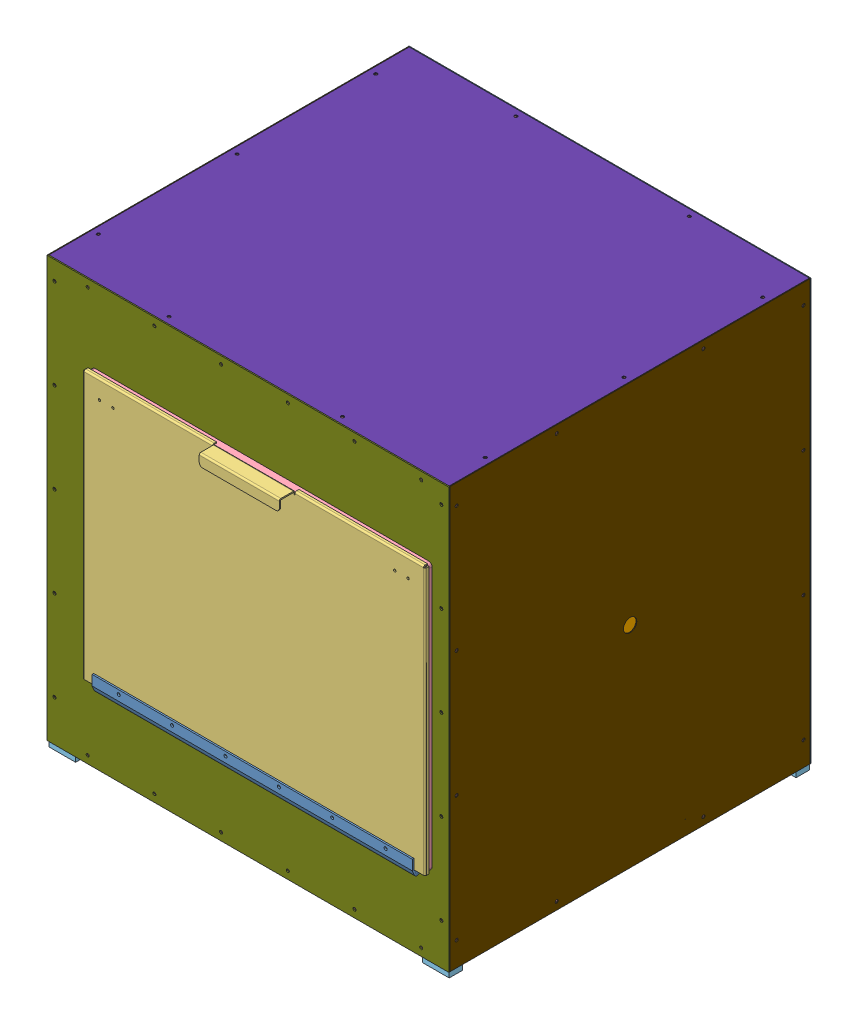
SolidWorks assembly Larva Tracker Assembly_Updated, configuration Default. Lengths in mm. (continued)
Components (placement in the parent): (continued)
- T-LSR450-5: T-LSR450 [Default] at (-127.5387 377.3527 -6.3502) x (0 0 1) z (1 0 0) size (65 43.34 637) (continued)
  - Bearing_Thrust_4-8-4-1: Bearing_Thrust_4-8-4 [Default] at (-37.0232 -30.3507 624.2355) size (9 9 4)
  - Bearing_Thrust_4-8-4-2: Bearing_Thrust_4-8-4 [Default] at (-37.0232 -30.3507 630.0355) size (9 9 4)
  - Screw_M3 x 5 Button Cap-1: Screw_M3 x 5 Button Cap [Default] at (-37.0232 -30.3507 631.3355) size (5.7 5.7 6.65)
  - T-LSR450 Base-1: T-LSR450 Base [Default] at (-69.5232 -52.7431 101.5355) size (65 27 520)
  - T-LSR450 Compression Bar-1: T-LSR450 Compression Bar [Default] at (-59.7393 -36.3047 101.5355) x (0.707107 0.707107 0) z (0 0 1) size (6.35 6.35 519.5)
  - T-LSR Bearing End Plate_Thrust Bearing Version1-1: T-LSR Bearing End Plate_Thrust Bearing Version1 [Default] at (-5.0232 -52.2431 633.5355) x (-1 0 0) z (0 0 -1) size (64 34.8 12)
  - Motor Mount End Plate-1: Motor Mount End Plate [Default] at (-69.0232 -52.2431 95.5355) size (64 42 6)
  - T-LSR450 Compression Bar-2: T-LSR450 Compression Bar [Default] at (-14.3071 -36.3047 101.5355) x (0.707107 0.707107 0) z (0 0 1) size (6.35 6.35 519.5)
  - Screw M3 x 8 SC-1: Screw M3 x 8 SC [Default] at (-8.5232 -48.7431 624.5355) size (5.5 5.5 11)
  - Screw M3 x 8 SC-2: Screw M3 x 8 SC [Default] at (-65.5232 -28.7431 624.5355) size (5.5 5.5 11)
  - Screw M3 x 8 SC-3: Screw M3 x 8 SC [Default] at (-8.5232 -28.7431 624.5355) size (5.5 5.5 11)
  - Screw M3 x 8 SC-4: Screw M3 x 8 SC [Default] at (-65.5232 -48.7431 624.5355) size (5.5 5.5 11)
  - Screw M3 x 8 SC-5: Screw M3 x 8 SC [Default] at (-21.5232 -14.8531 98.3355) size (5.5 5.5 11)
  - Screw M3 x 8 SC-6: Screw M3 x 8 SC [Default] at (-52.5232 -14.8531 98.3355) size (5.5 5.5 11)
  - Screw M3 x 8 SC-7: Screw M3 x 8 SC [Default] at (-21.5232 -45.8531 98.3355) size (5.5 5.5 11)
  - Screw M3 x 8 SC-8: Screw M3 x 8 SC [Default] at (-65.5232 -28.7431 98.5355) x (0.044892 0.998992 0) z (0 0 -1) size (5.5 5.5 11)
  - Screw M3 x 8 SC-9: Screw M3 x 8 SC [Default] at (-8.5232 -28.7431 98.5355) x (-0.436079 0.899908 0) z (0 0 -1) size (5.5 5.5 11)
  - Screw M3 x 8 SC-10: Screw M3 x 8 SC [Default] at (-8.5232 -48.7431 98.5355) x (0.383001 0.923748 0) z (0 0 -1) size (5.5 5.5 11)
  - Screw M3 x 8 SC-11: Screw M3 x 8 SC [Default] at (-65.5232 -48.7431 98.5355) x (0.453529 0.891241 0) z (0 0 -1) size (5.5 5.5 11)
  - Screw M3 x 8 SC-12: Screw M3 x 8 SC [Default] at (-52.5232 -45.8531 98.3355) size (5.5 5.5 11)
- Car sub assy-4: Car sub assy [Default] at (32.9968 407.7034 -43.3734) x (0 0 1) z (1 0 0) size (64 28.83 65.47)
  - Lead Screw Nut-1: Lead Screw Nut [Default] at origin size (22.86 20.6 25.4)
  - Screw_M3x12 CS-1: Screw_M3x12 CS [Default] at (8.2532 -4.765 4.546) size (5.92 5.92 12)
  - Screw_M3x12 CS-2: Screw_M3x12 CS [Default] at (-8.2532 -4.765 4.546) size (5.92 5.92 12)
  - Screw_M3x12 CS-3: Screw_M3x12 CS [Default] at (0 9.53 4.546) size (5.92 5.92 12)
  - Washer_5-32ID-1: Washer_5-32ID [Default] at (18.1354 5.1807 -52.75) x (0.633432 -0.633432 -0.44444) z (0.707107 0.707107 0) size (6.35 6.35 0.33)
  - Bearing Washer-1: Bearing Washer [Default] at (-18.3674 -8.3405 -0.25) x (0.5 -0.5 -0.707107) z (0.707107 0.707107 0) size (6.35 6.35 0.2)
  - 3%8 in bearing-1: 3%8 in bearing [Default] at (18.226 -8.199 -0.25) x (0.42856 0.42856 -0.795407) z (-0.707107 0.707107 0) size (9.53 9.53 3.17)
  - Bearing Washer-2: Bearing Washer [Default] at (15.9809 -5.954 -0.25) x (0.5 0.5 0.707107) z (-0.707107 0.707107 0) size (6.35 6.35 0.2)
  - Bearing Washer-3: Bearing Washer [Default] at (18.2273 5.2726 -8.75) x (0.5 -0.5 -0.707107) z (0.707107 0.707107 0) size (6.35 6.35 0.2)
  - 3%8 in bearing-2: 3%8 in bearing [Default] at (15.9822 3.0276 -8.75) x (0.5 -0.5 -0.707107) z (0.707107 0.707107 0) size (9.53 9.53 3.17)
  - 3%8 in bearing-3: 3%8 in bearing [Default] at (15.8903 2.9356 -52.75) x (0.65714 -0.65714 -0.369234) z (0.707107 0.707107 0) size (9.53 9.53 3.17)
  - ShoulderScrew-1: ShoulderScrew [Default] at (15.8903 2.9356 -52.75) x (0.530428 -0.530428 0.66128) z (-0.707107 -0.707107 0) size (7.95 7.95 13.65)
  - Bearing Washer-4: Bearing Washer [Default] at (15.9809 -5.954 -44.25) x (0.5 0.5 0.707107) z (-0.707107 0.707107 0) size (6.35 6.35 0.2)
  - 3%8 in bearing-4: 3%8 in bearing [Default] at (18.226 -8.199 -44.25) x (0.42856 0.42856 -0.795407) z (-0.707107 0.707107 0) size (9.53 9.53 3.17)
  - ShoulderScrew-2: ShoulderScrew [Default] at (18.226 -8.199 -44.25) x (0.405923 0.405923 -0.818812) z (0.707107 -0.707107 0) size (7.95 7.95 13.65)
  - ShoulderScrew-3: ShoulderScrew [Default] at (-18.226 -8.199 -44.25) x (0.498357 -0.498357 -0.709423) z (-0.707107 -0.707107 0) size (7.95 7.95 13.65)
  - ShoulderScrew-4: ShoulderScrew [Default] at (15.9822 3.0276 -8.75) x (0.496183 -0.496183 -0.712464) z (-0.707107 -0.707107 0) size (7.95 7.95 13.65)
  - Bearing Washer-5: Bearing Washer [Default] at (-15.9809 -5.954 -44.25) x (0.5 -0.5 -0.707107) z (0.707107 0.707107 0) size (6.35 6.35 0.2)
  - 3%8 in bearing-5: 3%8 in bearing [Default] at (-15.9809 -5.954 -44.25) x (-0.308196 0.308196 -0.900017) z (-0.707107 -0.707107 0) size (9.53 9.53 3.17)
  - Bearing Washer-6: Bearing Washer [Default] at (-18.3687 5.4141 -52.75) x (0.408741 0.408741 -0.816004) z (0.707107 -0.707107 0) size (6.35 6.35 0.2)
  - ShoulderScrew-5: ShoulderScrew [Default] at (-15.9822 3.0276 -52.75) x (0.451656 0.451656 -0.769424) z (0.707107 -0.707107 0) size (7.95 7.95 13.65)
  - 3%8 in bearing-6: 3%8 in bearing [Default] at (-18.2273 5.2726 -52.75) x (0.225478 0.225478 -0.947797) z (0.707107 -0.707107 0) size (9.53 9.53 3.17)
  - ShoulderScrew-6: ShoulderScrew [Default] at (18.226 -8.199 -0.25) x (0.471234 0.471234 -0.745572) z (0.707107 -0.707107 0) size (7.95 7.95 13.65)
  - Bearing Washer-7: Bearing Washer [Default] at (-15.9809 -5.954 -0.25) x (0.5 -0.5 -0.707107) z (0.707107 0.707107 0) size (6.35 6.35 0.2)
  - 3%8 in bearing-7: 3%8 in bearing [Default] at (-15.9809 -5.954 -0.25) x (-0.308196 0.308196 -0.900017) z (-0.707107 -0.707107 0) size (9.53 9.53 3.17)
  - Bearing Washer-8: Bearing Washer [Default] at (-18.2273 5.2726 -8.75) x (-0.44628 -0.44628 -0.775672) z (-0.707107 0.707107 0) size (6.35 6.35 0.2)
  - ShoulderScrew-7: ShoulderScrew [Default] at (-15.9822 3.0276 -8.75) x (-0.382714 -0.382714 -0.840868) z (0.707107 -0.707107 0) size (7.95 7.95 13.65)
  - 3%8 in bearing-8: 3%8 in bearing [Default] at (-18.2273 5.2726 -8.75) x (-0.663315 -0.663315 -0.34645) z (0.707107 -0.707107 0) size (9.53 9.53 3.17)
  - ShoulderScrew-8: ShoulderScrew [Default] at (-18.3674 -8.3405 -0.25) x (0.692139 -0.692139 0.204665) z (-0.707107 -0.707107 0) size (7.95 7.95 13.65)
  - T-LSR Top-1: T-LSR Top [Default] at (-23.2 -10.11 -59) size (64 23.75 65.05)
- Zaber Bracket_Flat-3: Zaber Bracket_Flat [Default] at (-33.5032 430.0958 -43.3734) size (127 6.35 65)
- Mini Series LED Assy-1: Mini Series LED Assy [Default] at (78.0588 375.5809 -14.1992) x (-0.5 0 -0.866025) z (-0.866025 0 0.5) size (47.25 137.87 73.84)
  - 8587-E0W-1: 8587-E0W [Default] at origin size (22.09 50.8 43.59)
  - 8579-E0W-1: 8579-E0W [Default] at (0.7035 47.0774 0.0339) x (0.960592 0 0.277963) z (-0.277963 0 0.960592) size (5.99 79.38 5.99)
  - 13441-E0W-1: 13441-E0W [One Thumbscrew] at (12.7 76.5797 12.7) x (0 0 -1) z (1 0 0) size (26.9 12.7 12.7)
  - 13441-E0W-2: 13441-E0W [Default] at (12.7 72.1347 8.255) x (0 1 0) z (1 0 0) size (34.75 12.7 13.61)
  - 11899-E0W-1: 11899-E0W [Default] at (12.7 68.3247 24.257) x (0 0 -1) z (0.815203 -0.579175 0) size (12.7 10.16 10.16)
  - 8573-E0W-1: 8573-E0W [Default] at (13.2183 68.8017 7.9627) x (0.872563 0.488502 0) z (0.488502 -0.872563 0) size (5.99 28.57 5.99)
  - Mightex LED Assy-1: Mightex LED Assy [Default] at (12.6968 29.4075 40.543) x (0 0 1) z (-1 0 0) size (39.47 104.26 40.73)
    - Mightex_LED-1: Mightex_LED [Default] at origin size (28 88.76 35)
    - Mightex_Focusing Module-1: Mightex_Focusing Module [Default] at (0 104.26 0) x (-0.598321 0 0.801257) z (0.801257 0 0.598321) size (28.2 20.5 28.2)
- Mini Series LED Assy-2: Mini Series LED Assy [Default] at (-52.9588 375.5809 -36.1906) x (-0.5 0 0.866025) z (0.866025 0 0.5) size (47.25 137.87 73.84)
  - 8587-E0W-1: 8587-E0W [Default] at origin size (22.09 50.8 43.59)
  - 8579-E0W-1: 8579-E0W [Default] at (0.7035 47.0774 0.0339) x (0.960592 0 0.277963) z (-0.277963 0 0.960592) size (5.99 79.38 5.99)
  - 13441-E0W-1: 13441-E0W [One Thumbscrew] at (12.7 76.5797 12.7) x (0 0 -1) z (1 0 0) size (26.9 12.7 12.7)
  - 13441-E0W-2: 13441-E0W [Default] at (12.7 72.1347 8.255) x (0 1 0) z (1 0 0) size (34.75 12.7 13.61)
  - 11899-E0W-1: 11899-E0W [Default] at (12.7 68.3247 24.257) x (0 0 -1) z (0.815203 -0.579175 0) size (12.7 10.16 10.16)
  - 8573-E0W-1: 8573-E0W [Default] at (13.2183 68.8017 7.9627) x (0.872563 0.488502 0) z (0.488502 -0.872563 0) size (5.99 28.57 5.99)
  - Mightex LED Assy-1: Mightex LED Assy [Default] at (12.6968 29.4075 40.543) x (0 0 1) z (-1 0 0) size (39.47 104.26 40.73)
    - Mightex_LED-1: Mightex_LED [Default] at origin size (28 88.76 35)
    - Mightex_Focusing Module-1: Mightex_Focusing Module [Default] at (0 104.26 0) x (-0.598321 0 0.801257) z (0.801257 0 0.598321) size (28.2 20.5 28.2)
- Mini Series LED Assy-3: Mini Series LED Assy [Default] at (-6.4952 375.5809 88.2696) x (1 0 0) z (0 0 -1) size (47.25 137.87 73.84)
  - 8587-E0W-1: 8587-E0W [Default] at origin size (22.09 50.8 43.59)
  - 8579-E0W-1: 8579-E0W [Default] at (0.7035 47.0774 0.0339) x (0.960592 0 0.277963) z (-0.277963 0 0.960592) size (5.99 79.38 5.99)
  - 13441-E0W-1: 13441-E0W [One Thumbscrew] at (12.7 76.5797 12.7) x (0 0 -1) z (1 0 0) size (26.9 12.7 12.7)
  - 13441-E0W-2: 13441-E0W [Default] at (12.7 72.1347 8.255) x (0 1 0) z (1 0 0) size (34.75 12.7 13.61)
  - 11899-E0W-1: 11899-E0W [Default] at (12.7 68.3247 24.257) x (0 0 -1) z (0.815203 -0.579175 0) size (12.7 10.16 10.16)
  - 8573-E0W-1: 8573-E0W [Default] at (13.2183 68.8017 7.9627) x (0.872563 0.488502 0) z (0.488502 -0.872563 0) size (5.99 28.57 5.99)
  - Mightex LED Assy-1: Mightex LED Assy [Default] at (12.6968 29.4075 40.543) x (0 0 1) z (-1 0 0) size (39.47 104.26 40.73)
    - Mightex_LED-1: Mightex_LED [Default] at origin size (28 88.76 35)
    - Mightex_Focusing Module-1: Mightex_Focusing Module [Default] at (0 104.26 0) x (-0.598321 0 0.801257) z (0.801257 0 0.598321) size (28.2 20.5 28.2)
- Zaber Bracket-4: Zaber Bracket [Stepped] at (504.2268 430.0958 -43.3734) size (107.95 18.13 65)
- THK Rail-2: THK Rail [Default] at (525.9968 472.2282 -294.9174) x (0 0 1) z (1 0 0) size (538 12.5 15)
- THK car-4: THK car [Default] at (525.9968 472.2282 226.6266) x (0 0 -1) z (-1 0 0) size (60.5 19.5 34)
  - grease plug-1: grease plug [Default] at (540 0.1661 2.4399) x (-1 0 0) z (0 -0.135551 -0.99077) size (9.5 7.5 7.5)
  - THK SR-15W-1: THK SR-15W [Default] at origin size (57 19.5 34)
- LED Plate-1: LED Plate [Default] at (6.4968 386.0584 -43.3734) size (166.79 14.61 177.51)
- Edmund_NT63-977-1: Edmund_NT63-977 [Default] at (-7.3434 518.4647 22.1417) x (-1 0 0) z (0 -1 0) size (56.02 47.95 12.7)
- Camera Bracket_3-1: Camera Bracket_3 [Default] at (6.2016 580.953 36.6516) x (1 0 0) z (0 1 0) size (44 13.56 213.75)
- Thor Lab MS1 stage 6132-E0W-1: Thor Lab MS1 stage 6132-E0W [Default] at (6.2016 463.538 43.6046) x (1 0 0) z (0 -1 0) size (30.81 15.24 58.61)
- Camera Bracket-1: Camera Bracket [Default] at (-27.8634 386.0584 24.8086) x (-1 0 0) z (0 0 -1) size (58.45 92.34 53.34)
- Rexroth-8 981 021 399_-1: Rexroth-8 981 021 399_ [23 in lg] at (0 -39.6993 5.2) x (0 -1 0) z (0 0 1) size (25.4 50.8 584.2)
- Rexroth-8 981 021 399_-2: Rexroth-8 981 021 399_ [30 in lg no holes] at (206.0409 -39.6993 -312.3013) x (0 1 0) z (-1 0 0) size (25.4 50.8 762)
- Rexroth-8 981 021 399_-3: Rexroth-8 981 021 399_ [23 in lg] at (495.2935 -39.6993 5.2) x (0 -1 0) z (0 0 1) size (25.4 50.8 584.2)
- Rexroth-8 981 021 399_-4: Rexroth-8 981 021 399_ [23 in lg] at (-149.5604 -39.6993 5.1974) x (0 -1 0) z (0 0 1) size (25.4 50.8 584.2)
- Rexroth-8 981 021 399_-6: Rexroth-8 981 021 399_ [30.375 in lg] at (-162.2597 358.7625 322.6987) x (1 0 0) z (0 -1 0) size (25.4 50.8 771.52)
- Rexroth-8 981 021 399_-7: Rexroth-8 981 021 399_ [30 in lg no holes] at (206.0409 -39.6993 322.6987) x (0 1 0) z (-1 0 0) size (25.4 50.8 762)
- Rexroth-8 981 021 399_-8: Rexroth-8 981 021 399_ [23 in lg] at (-65.0032 484.9276 5.2) x (0 1 0) z (0 0 1) size (25.4 50.8 584.2)
- Rexroth-8 981 021 399_-9: Rexroth-8 981 021 399_ [23 in lg] at (538.6962 484.9276 5.2) x (0 1 0) z (0 0 1) size (25.4 50.8 584.2)
- Rexroth-8 981 021 399_-10: Rexroth-8 981 021 399_ [30.375 in lg] at (574.3403 358.7625 322.6987) x (1 0 0) z (0 -1 0) size (25.4 50.8 771.52)
- Rexroth-8 981 021 399_-11: Rexroth-8 981 021 399_ [30.375 in lg] at (-162.2597 358.7625 -312.3013) x (1 0 0) z (0 -1 0) size (25.4 50.8 771.52)
- Rexroth-8 981 021 399_-12: Rexroth-8 981 021 399_ [30.375 in lg] at (574.3403 358.7625 -312.3013) x (1 0 0) z (0 -1 0) size (25.4 50.8 771.52)
- Rexroth-8 981 021 399_-13: Rexroth-8 981 021 399_ [28 in lg] at (206.0396 108.564 322.6987) x (0 -1 0) z (1 0 0) size (25.4 50.8 711.2)
- Rexroth-8 981 021 399_-14: Rexroth-8 981 021 399_ [28 in lg] at (206.0396 108.564 -312.3013) x (0 -1 0) z (1 0 0) size (25.4 50.8 711.2)
- Rexroth-8 981 021 399_-15: Rexroth-8 981 021 399_ [28 in lg] at (206.0396 484.9276 322.6987) x (0 -1 0) z (-1 0 0) size (25.4 50.8 711.2)
- Rexroth-8 981 021 399_-16: Rexroth-8 981 021 399_ [28 in lg] at (206.0396 484.9276 -312.3013) x (0 -1 0) z (-1 0 0) size (25.4 50.8 711.2)
- Rexroth-8 981 021 399_-17: Rexroth-8 981 021 399_ [28 in lg] at (206.0396 731.8383 322.6987) x (0 -1 0) z (-1 0 0) size (25.4 50.8 711.2)
- Rexroth-8 981 021 399_-18: Rexroth-8 981 021 399_ [28 in lg] at (206.0396 731.8383 -312.3013) x (0 -1 0) z (-1 0 0) size (25.4 50.8 711.2)
- Rexroth-8 981 021 399_-19: Rexroth-8 981 021 399_ [23 in lg] at (-149.5604 731.8257 5.1974) x (0 -1 0) z (0 0 1) size (25.4 50.8 584.2)
- Rexroth-8 981 021 399_-20: Rexroth-8 981 021 399_ [23 in lg] at (561.6396 731.8257 5.1974) x (0 -1 0) z (0 0 1) size (25.4 50.8 584.2)
- Back Sheet -1: Back Sheet  [Default] at (586.0871 -51.4462 -337.7) x (0 -1 0) z (0 0 1) size (800.1 765.17 1.59)
- Bottom Sheet -1: Bottom Sheet  [Default] at (587.0396 -52.3987 348.1) size (762 1.59 685.8)
- Front Sheet -1: Front Sheet  [Default] at (-176.5466 -53.9862 348.0974) x (0 -1 0) z (0 0 -1) size (800.1 765.17 2.29)
- Top Sheet -1: Top Sheet  [Default] at (-174.9604 744.525 348.0968) x (-1 0 0) z (0 0 1) size (762 1.59 685.8)
- Side Sheet -1: Side Sheet  [Default] at (-174.9591 -53.9862 -337.7) x (-1 0 0) z (0 -1 0) size (1.59 685.8 800.1)
- Side Sheet -2: Side Sheet  [Default] at (588.6271 -53.9862 -337.7) x (-1 0 0) z (0 -1 0) size (1.59 685.8 800.1)
- 1581A167_Hinge-1: 1581A167_Hinge [closed] at (-376.844 91.0253 351.9074) x (0 -1 0) z (-1 0 0) size (50.8 18.54 609.6)
- 1745A12_bracket-4: 1745A12_bracket [Default] at (-48.1572 572.5617 361.153) x (0 1 0) z (1 0 0) size (15.08 1.2 34.92)
- Door Assembly-1: Door Assembly [Default] at (6.0918 195.2159 -419.4229) size (652.27 510.63 43.18)
  - Door-1: Door [Default] at (-97.1115 -97.7136 783.0143) x (0 0 1) z (0 -1 0) size (35.05 652.27 510.29)
  - Door Gasket-1: Door Gasket [Default] at (226.7408 155.9442 783.0143) size (647.7 508 13.21)
- T-LSR450-6: T-LSR450 [Default] at (37.02 25.7431 -379.7755) size (65 43.34 637)
  - NM17-H-1: NM17-H [Default] at (-58.1732 -51.5031 48.5355) size (42.1 42.1 71.3)
  - T-NM17 Housing-1: T-NM17 Housing [Default] at (-16.1232 -51.2531 48.5355) x (-1 0 0) z (0 0 -1) size (41.8 41.8 52)
  - knob_LA-1: knob_LA [Default] at (-37.2232 -26.0531 -6.7645) (suppressed, hidden)
  - Coupling_CPS12-1: Coupling_CPS12 [Default] at (-37.0232 -30.3531 128.8355) x (0.334969 -0.942229 0) z (0 0 -1) size (12 12 14)
  - Car sub assy-1: Car sub assy [Default] at (-37.0232 -30.3531 234.0931) size (64 28.83 65.47) (suppressed, hidden)
    - Lead Screw Nut-1: Lead Screw Nut [Default] at origin size (22.86 20.6 25.4)
    - Screw_M3x12 CS-1: Screw_M3x12 CS [Default] at (8.2532 -4.765 4.546) size (5.92 5.92 12)
    - Screw_M3x12 CS-2: Screw_M3x12 CS [Default] at (-8.2532 -4.765 4.546) size (5.92 5.92 12)
    - Screw_M3x12 CS-3: Screw_M3x12 CS [Default] at (0 9.53 4.546) size (5.92 5.92 12)
    - Washer_5-32ID-1: Washer_5-32ID [Default] at (18.1354 5.1807 -52.75) x (0.633432 -0.633432 -0.44444) z (0.707107 0.707107 0) size (6.35 6.35 0.33)
    - Bearing Washer-1: Bearing Washer [Default] at (-18.3674 -8.3405 -0.25) x (0.5 -0.5 -0.707107) z (0.707107 0.707107 0) size (6.35 6.35 0.2)
    - 3%8 in bearing-1: 3%8 in bearing [Default] at (18.226 -8.199 -0.25) x (0.42856 0.42856 -0.795407) z (-0.707107 0.707107 0) size (9.53 9.53 3.17)
    - Bearing Washer-2: Bearing Washer [Default] at (15.9809 -5.954 -0.25) x (0.5 0.5 0.707107) z (-0.707107 0.707107 0) size (6.35 6.35 0.2)
    - Bearing Washer-3: Bearing Washer [Default] at (18.2273 5.2726 -8.75) x (0.5 -0.5 -0.707107) z (0.707107 0.707107 0) size (6.35 6.35 0.2)
    - 3%8 in bearing-2: 3%8 in bearing [Default] at (15.9822 3.0276 -8.75) x (0.5 -0.5 -0.707107) z (0.707107 0.707107 0) size (9.53 9.53 3.17)
    - 3%8 in bearing-3: 3%8 in bearing [Default] at (15.8903 2.9356 -52.75) x (0.65714 -0.65714 -0.369234) z (0.707107 0.707107 0) size (9.53 9.53 3.17)
    - ShoulderScrew-1: ShoulderScrew [Default] at (15.8903 2.9356 -52.75) x (0.530428 -0.530428 0.66128) z (-0.707107 -0.707107 0) size (7.95 7.95 13.65)
    - Bearing Washer-4: Bearing Washer [Default] at (15.9809 -5.954 -44.25) x (0.5 0.5 0.707107) z (-0.707107 0.707107 0) size (6.35 6.35 0.2)
    - 3%8 in bearing-4: 3%8 in bearing [Default] at (18.226 -8.199 -44.25) x (0.42856 0.42856 -0.795407) z (-0.707107 0.707107 0) size (9.53 9.53 3.17)
    - ShoulderScrew-2: ShoulderScrew [Default] at (18.226 -8.199 -44.25) x (0.405923 0.405923 -0.818812) z (0.707107 -0.707107 0) size (7.95 7.95 13.65)
    - ShoulderScrew-3: ShoulderScrew [Default] at (-18.226 -8.199 -44.25) x (0.498357 -0.498357 -0.709423) z (-0.707107 -0.707107 0) size (7.95 7.95 13.65)
    - ShoulderScrew-4: ShoulderScrew [Default] at (15.9822 3.0276 -8.75) x (0.496183 -0.496183 -0.712464) z (-0.707107 -0.707107 0) size (7.95 7.95 13.65)
    - Bearing Washer-5: Bearing Washer [Default] at (-15.9809 -5.954 -44.25) x (0.5 -0.5 -0.707107) z (0.707107 0.707107 0) size (6.35 6.35 0.2)
    - 3%8 in bearing-5: 3%8 in bearing [Default] at (-15.9809 -5.954 -44.25) x (-0.308196 0.308196 -0.900017) z (-0.707107 -0.707107 0) size (9.53 9.53 3.17)
    - Bearing Washer-6: Bearing Washer [Default] at (-18.3687 5.4141 -52.75) x (0.408741 0.408741 -0.816004) z (0.707107 -0.707107 0) size (6.35 6.35 0.2)
    - ShoulderScrew-5: ShoulderScrew [Default] at (-15.9822 3.0276 -52.75) x (0.451656 0.451656 -0.769424) z (0.707107 -0.707107 0) size (7.95 7.95 13.65)
    - 3%8 in bearing-6: 3%8 in bearing [Default] at (-18.2273 5.2726 -52.75) x (0.225478 0.225478 -0.947797) z (0.707107 -0.707107 0) size (9.53 9.53 3.17)
    - ShoulderScrew-6: ShoulderScrew [Default] at (18.226 -8.199 -0.25) x (0.471234 0.471234 -0.745572) z (0.707107 -0.707107 0) size (7.95 7.95 13.65)
    - Bearing Washer-7: Bearing Washer [Default] at (-15.9809 -5.954 -0.25) x (0.5 -0.5 -0.707107) z (0.707107 0.707107 0) size (6.35 6.35 0.2)
    - 3%8 in bearing-7: 3%8 in bearing [Default] at (-15.9809 -5.954 -0.25) x (-0.308196 0.308196 -0.900017) z (-0.707107 -0.707107 0) size (9.53 9.53 3.17)
    - Bearing Washer-8: Bearing Washer [Default] at (-18.2273 5.2726 -8.75) x (-0.44628 -0.44628 -0.775672) z (-0.707107 0.707107 0) size (6.35 6.35 0.2)
    - ShoulderScrew-7: ShoulderScrew [Default] at (-15.9822 3.0276 -8.75) x (-0.382714 -0.382714 -0.840868) z (0.707107 -0.707107 0) size (7.95 7.95 13.65)
    - 3%8 in bearing-8: 3%8 in bearing [Default] at (-18.2273 5.2726 -8.75) x (-0.663315 -0.663315 -0.34645) z (0.707107 -0.707107 0) size (9.53 9.53 3.17)
    - ShoulderScrew-8: ShoulderScrew [Default] at (-18.3674 -8.3405 -0.25) x (0.692139 -0.692139 0.204665) z (-0.707107 -0.707107 0) size (7.95 7.95 13.65)
    - T-LSR Top-1: T-LSR Top [Default] at (-23.2 -10.11 -59) size (64 23.75 65.05)
  - T-LSR450 Lead Screw-1: T-LSR450 Lead Screw [Default] at (-37.0232 -30.3507 123.8355) x (0.360518 -0.932752 0) z (0 0 1) size (6.34 6.34 506.7)
  - Screw M3 x 6 set screw-1: Screw M3 x 6 set screw [Default] at (-11.9381 -34.2188 486.5355) x (0.680208 0.680208 -0.273191) z (0.707107 -0.707107 0) size (3 3 6)
  - Screw M3 x 6 set screw-2: Screw M3 x 6 set screw [Default] at (-11.9381 -34.2188 461.5355) x (0.680208 0.680208 -0.273191) z (0.707107 -0.707107 0) size (3 3 6)
  - Screw M3 x 6 set screw-3: Screw M3 x 6 set screw [Default] at (-11.9381 -34.2188 436.5355) x (0.680208 0.680208 -0.273191) z (0.707107 -0.707107 0) size (3 3 6)
  - Screw M3 x 6 set screw-4: Screw M3 x 6 set screw [Default] at (-62.1082 -34.2188 461.5355) x (0.146534 -0.146534 0.978292) z (-0.707107 -0.707107 0) size (3 3 6)
  - Screw M3 x 6 set screw-5: Screw M3 x 6 set screw [Default] at (-62.1082 -34.2188 436.5355) x (0.289314 -0.289314 0.912466) z (-0.707107 -0.707107 0) size (3 3 6)
  - Screw M3 x 6 set screw-6: Screw M3 x 6 set screw [Default] at (-11.9381 -34.2188 536.5355) x (0.680208 0.680208 -0.273191) z (0.707107 -0.707107 0) size (3 3 6)
  - Screw M3 x 6 set screw-7: Screw M3 x 6 set screw [Default] at (-62.1082 -34.2188 411.5355) x (0.704993 -0.704993 0.077261) z (-0.707107 -0.707107 0) size (3 3 6)
  - Screw M3 x 6 set screw-8: Screw M3 x 6 set screw [Default] at (-11.9381 -34.2188 561.5355) x (0.680208 0.680208 -0.273191) z (0.707107 -0.707107 0) size (3 3 6)
  - Screw M3 x 6 set screw-9: Screw M3 x 6 set screw [Default] at (-11.9381 -34.2188 511.5355) x (0.680208 0.680208 -0.273191) z (0.707107 -0.707107 0) size (3 3 6)
  - Screw M3 x 6 set screw-10: Screw M3 x 6 set screw [Default] at (-62.1082 -34.2188 486.5355) x (0.67969 -0.67969 0.275758) z (-0.707107 -0.707107 0) size (3 3 6)
  - Screw M3 x 6 set screw-11: Screw M3 x 6 set screw [Default] at (-62.1082 -34.2188 511.5355) x (-0.395154 0.395154 -0.829281) z (-0.707107 -0.707107 0) size (3 3 6)
  - Screw M3 x 6 set screw-12: Screw M3 x 6 set screw [Default] at (-62.1082 -34.2188 561.5355) x (-0.551643 0.551643 -0.625603) z (-0.707107 -0.707107 0) size (3 3 6)
  - Screw M3 x 6 set screw-13: Screw M3 x 6 set screw [Default] at (-62.1082 -34.2188 536.5355) x (-0.617589 0.617589 -0.486998) z (-0.707107 -0.707107 0) size (3 3 6)
  - Screw M3 x 6 set screw-14: Screw M3 x 6 set screw [Default] at (-11.9381 -34.2188 586.5355) x (0.680208 0.680208 -0.273191) z (0.707107 -0.707107 0) size (3 3 6)
  - Screw M3 x 6 set screw-15: Screw M3 x 6 set screw [Default] at (-62.1082 -34.2188 611.5355) x (-0.585905 0.585905 -0.559849) z (-0.707107 -0.707107 0) size (3 3 6)
  - Screw M3 x 6 set screw-16: Screw M3 x 6 set screw [Default] at (-62.1082 -34.2188 586.5355) x (-0.690783 0.690783 -0.213627) z (-0.707107 -0.707107 0) size (3 3 6)
  - Screw M3 x 6 set screw-17: Screw M3 x 6 set screw [Default] at (-11.9381 -34.2188 611.5355) x (0.680208 0.680208 -0.273191) z (0.707107 -0.707107 0) size (3 3 6)
  - Screw M3 x 6 set screw-18: Screw M3 x 6 set screw [Default] at (-11.9381 -34.2188 411.5355) x (0.680208 0.680208 -0.273191) z (0.707107 -0.707107 0) size (3 3 6)
  - Bearing_Thrust_4-8-4-1: Bearing_Thrust_4-8-4 [Default] at (-37.0232 -30.3507 624.2355) size (9 9 4)
  - Bearing_Thrust_4-8-4-2: Bearing_Thrust_4-8-4 [Default] at (-37.0232 -30.3507 630.0355) size (9 9 4)
  - Screw_M3 x 5 Button Cap-1: Screw_M3 x 5 Button Cap [Default] at (-37.0232 -30.3507 631.3355) size (5.7 5.7 6.65)
  - T-LSR450 Base-1: T-LSR450 Base [Default] at (-69.5232 -52.7431 101.5355) size (65 27 520)
  - T-LSR450 Compression Bar-1: T-LSR450 Compression Bar [Default] at (-59.7393 -36.3047 101.5355) x (0.707107 0.707107 0) z (0 0 1) size (6.35 6.35 519.5)
  - T-LSR Bearing End Plate_Thrust Bearing Version1-1: T-LSR Bearing End Plate_Thrust Bearing Version1 [Default] at (-5.0232 -52.2431 633.5355) x (-1 0 0) z (0 0 -1) size (64 34.8 12)
  - Motor Mount End Plate-1: Motor Mount End Plate [Default] at (-69.0232 -52.2431 95.5355) size (64 42 6)
  - T-LSR450 Compression Bar-2: T-LSR450 Compression Bar [Default] at (-14.3071 -36.3047 101.5355) x (0.707107 0.707107 0) z (0 0 1) size (6.35 6.35 519.5)
  - Screw M3 x 8 SC-1: Screw M3 x 8 SC [Default] at (-8.5232 -48.7431 624.5355) size (5.5 5.5 11)
  - Screw M3 x 8 SC-2: Screw M3 x 8 SC [Default] at (-65.5232 -28.7431 624.5355) size (5.5 5.5 11)
  - Screw M3 x 8 SC-3: Screw M3 x 8 SC [Default] at (-8.5232 -28.7431 624.5355) size (5.5 5.5 11)
  - Screw M3 x 8 SC-4: Screw M3 x 8 SC [Default] at (-65.5232 -48.7431 624.5355) size (5.5 5.5 11)
  - Screw M3 x 8 SC-5: Screw M3 x 8 SC [Default] at (-21.5232 -14.8531 98.3355) size (5.5 5.5 11)
  - Screw M3 x 8 SC-6: Screw M3 x 8 SC [Default] at (-52.5232 -14.8531 98.3355) size (5.5 5.5 11)
  - Screw M3 x 8 SC-7: Screw M3 x 8 SC [Default] at (-21.5232 -45.8531 98.3355) size (5.5 5.5 11)
  - Screw M3 x 8 SC-8: Screw M3 x 8 SC [Default] at (-65.5232 -28.7431 98.5355) x (0.044892 0.998992 0) z (0 0 -1) size (5.5 5.5 11)
  - Screw M3 x 8 SC-9: Screw M3 x 8 SC [Default] at (-8.5232 -28.7431 98.5355) x (-0.436079 0.899908 0) z (0 0 -1) size (5.5 5.5 11)
  - Screw M3 x 8 SC-10: Screw M3 x 8 SC [Default] at (-8.5232 -48.7431 98.5355) x (0.383001 0.923748 0) z (0 0 -1) size (5.5 5.5 11)
  - Screw M3 x 8 SC-11: Screw M3 x 8 SC [Default] at (-65.5232 -48.7431 98.5355) x (0.453529 0.891241 0) z (0 0 -1) size (5.5 5.5 11)
  - Screw M3 x 8 SC-12: Screw M3 x 8 SC [Default] at (-52.5232 -45.8531 98.3355) size (5.5 5.5 11)
- Car sub assy-5: Car sub assy [Default] at (-0.0032 -4.6076 23.8866) size (64 28.83 65.47)
  - Lead Screw Nut-1: Lead Screw Nut [Default] at origin size (22.86 20.6 25.4)
  - Screw_M3x12 CS-1: Screw_M3x12 CS [Default] at (8.2532 -4.765 4.546) size (5.92 5.92 12)
  - Screw_M3x12 CS-2: Screw_M3x12 CS [Default] at (-8.2532 -4.765 4.546) size (5.92 5.92 12)
  - Screw_M3x12 CS-3: Screw_M3x12 CS [Default] at (0 9.53 4.546) size (5.92 5.92 12)
  - Washer_5-32ID-1: Washer_5-32ID [Default] at (18.1354 5.1807 -52.75) x (0.633432 -0.633432 -0.44444) z (0.707107 0.707107 0) size (6.35 6.35 0.33)
  - Bearing Washer-1: Bearing Washer [Default] at (-18.3674 -8.3405 -0.25) x (0.5 -0.5 -0.707107) z (0.707107 0.707107 0) size (6.35 6.35 0.2)
  - 3%8 in bearing-1: 3%8 in bearing [Default] at (18.226 -8.199 -0.25) x (0.42856 0.42856 -0.795407) z (-0.707107 0.707107 0) size (9.53 9.53 3.17)
  - Bearing Washer-2: Bearing Washer [Default] at (15.9809 -5.954 -0.25) x (0.5 0.5 0.707107) z (-0.707107 0.707107 0) size (6.35 6.35 0.2)
  - Bearing Washer-3: Bearing Washer [Default] at (18.2273 5.2726 -8.75) x (0.5 -0.5 -0.707107) z (0.707107 0.707107 0) size (6.35 6.35 0.2)
  - 3%8 in bearing-2: 3%8 in bearing [Default] at (15.9822 3.0276 -8.75) x (0.5 -0.5 -0.707107) z (0.707107 0.707107 0) size (9.53 9.53 3.17)
  - 3%8 in bearing-3: 3%8 in bearing [Default] at (15.8903 2.9356 -52.75) x (0.65714 -0.65714 -0.369234) z (0.707107 0.707107 0) size (9.53 9.53 3.17)
  - ShoulderScrew-1: ShoulderScrew [Default] at (15.8903 2.9356 -52.75) x (0.530428 -0.530428 0.66128) z (-0.707107 -0.707107 0) size (7.95 7.95 13.65)
  - Bearing Washer-4: Bearing Washer [Default] at (15.9809 -5.954 -44.25) x (0.5 0.5 0.707107) z (-0.707107 0.707107 0) size (6.35 6.35 0.2)
  - 3%8 in bearing-4: 3%8 in bearing [Default] at (18.226 -8.199 -44.25) x (0.42856 0.42856 -0.795407) z (-0.707107 0.707107 0) size (9.53 9.53 3.17)
  - ShoulderScrew-2: ShoulderScrew [Default] at (18.226 -8.199 -44.25) x (0.405923 0.405923 -0.818812) z (0.707107 -0.707107 0) size (7.95 7.95 13.65)
  - ShoulderScrew-3: ShoulderScrew [Default] at (-18.226 -8.199 -44.25) x (0.498357 -0.498357 -0.709423) z (-0.707107 -0.707107 0) size (7.95 7.95 13.65)
  - ShoulderScrew-4: ShoulderScrew [Default] at (15.9822 3.0276 -8.75) x (0.496183 -0.496183 -0.712464) z (-0.707107 -0.707107 0) size (7.95 7.95 13.65)
  - Bearing Washer-5: Bearing Washer [Default] at (-15.9809 -5.954 -44.25) x (0.5 -0.5 -0.707107) z (0.707107 0.707107 0) size (6.35 6.35 0.2)
  - 3%8 in bearing-5: 3%8 in bearing [Default] at (-15.9809 -5.954 -44.25) x (-0.308196 0.308196 -0.900017) z (-0.707107 -0.707107 0) size (9.53 9.53 3.17)
  - Bearing Washer-6: Bearing Washer [Default] at (-18.3687 5.4141 -52.75) x (0.408741 0.408741 -0.816004) z (0.707107 -0.707107 0) size (6.35 6.35 0.2)
  - ShoulderScrew-5: ShoulderScrew [Default] at (-15.9822 3.0276 -52.75) x (0.451656 0.451656 -0.769424) z (0.707107 -0.707107 0) size (7.95 7.95 13.65)
  - 3%8 in bearing-6: 3%8 in bearing [Default] at (-18.2273 5.2726 -52.75) x (0.225478 0.225478 -0.947797) z (0.707107 -0.707107 0) size (9.53 9.53 3.17)
  - ShoulderScrew-6: ShoulderScrew [Default] at (18.226 -8.199 -0.25) x (0.471234 0.471234 -0.745572) z (0.707107 -0.707107 0) size (7.95 7.95 13.65)
  - Bearing Washer-7: Bearing Washer [Default] at (-15.9809 -5.954 -0.25) x (0.5 -0.5 -0.707107) z (0.707107 0.707107 0) size (6.35 6.35 0.2)
  - 3%8 in bearing-7: 3%8 in bearing [Default] at (-15.9809 -5.954 -0.25) x (-0.308196 0.308196 -0.900017) z (-0.707107 -0.707107 0) size (9.53 9.53 3.17)
  - Bearing Washer-8: Bearing Washer [Default] at (-18.2273 5.2726 -8.75) x (-0.44628 -0.44628 -0.775672) z (-0.707107 0.707107 0) size (6.35 6.35 0.2)
  - ShoulderScrew-7: ShoulderScrew [Default] at (-15.9822 3.0276 -8.75) x (-0.382714 -0.382714 -0.840868) z (0.707107 -0.707107 0) size (7.95 7.95 13.65)
  - 3%8 in bearing-8: 3%8 in bearing [Default] at (-18.2273 5.2726 -8.75) x (-0.663315 -0.663315 -0.34645) z (0.707107 -0.707107 0) size (9.53 9.53 3.17)
  - ShoulderScrew-8: ShoulderScrew [Default] at (-18.3674 -8.3405 -0.25) x (0.692139 -0.692139 0.204665) z (-0.707107 -0.707107 0) size (7.95 7.95 13.65)
  - T-LSR Top-1: T-LSR Top [Default] at (-23.2 -10.11 -59) size (64 23.75 65.05)
- 8020_2128-1: 8020_2128 [Default] at (561.6409 -52.3987 335.3974) x (0 0 -1) z (-1 0 0) size (25.4 12.7 50.8)
- 8020_2128-2: 8020_2128 [Default] at (-149.5591 -52.3987 335.3974) x (0 0 -1) z (-1 0 0) size (25.4 12.7 50.8)
- 8020_2128-3: 8020_2128 [Default] at (561.6409 -52.3987 -325.0026) x (0 0 -1) z (-1 0 0) size (25.4 12.7 50.8)
- 8020_2128-4: 8020_2128 [Default] at (-149.5591 -52.3987 -325.0026) x (0 0 -1) z (-1 0 0) size (25.4 12.7 50.8)
- Spacer Block-1: Spacer Block [Default] at (-48.1572 572.5617 361.153) x (1 0 0) z (0 1 0) size (34.92 10.77 15.08)
- Spacer Block-2: Spacer Block [Default] at (513.8201 572.5617 361.153) x (1 0 0) z (0 1 0) size (34.92 10.77 15.08)
- 1745A12_bracket-6: 1745A12_bracket [Default] at (513.8201 572.5617 361.153) x (0 1 0) z (1 0 0) size (15.08 1.2 34.92)
- 1745A12_magnet-7: 1745A12_magnet [Default] at (-48.1572 572.5617 361.607) x (0 1 0) z (1 0 0) size (11.91 1.98 34.92)
- 1745A12_magnet-8: 1745A12_magnet [Default] at (513.8201 572.5617 361.607) x (0 1 0) z (1 0 0) size (11.91 1.98 34.92)
- Rexroth-8 981 021 399_-21: Rexroth-8 981 021 399_ [23 in lg] at (574.3403 -27 5.2) size (25.4 50.8 584.2)
Mates (geometry in assembly coordinates):
- Concentric2: concentric anti-aligned: circle of T-LSR450-2/T-LSR450 Lead Screw-1; cylinder of Car sub assy-2/Lead Screw Nut-1 through (0.5668 31.1749 -2.6134) axis (-1 0 0) radius 3.175
- Parallel3: parallel aligned: plane of T-LSR450-2/T-LSR450 Base-1 through (-26.0032 35.7824 29.8866) normal (0 1 0); plane of Car sub assy-2/T-LSR Top-1 through (38.9968 44.5649 -34.6134) normal (0 1 0)
- Coincident15: coincident aligned: plane of T-LSR450-2/T-LSR450 Base-1 through (493.9968 8.7824 29.8866) normal (0 0 1); plane of Bottom Slider Bracket-1 through (440.4968 8.7824 29.8866) normal (0 0 1)
- Coincident191: coincident aligned: plane of T-LSR450-2/T-LSR Bearing End Plate_Thrust Bearing Version1-1 through (505.4968 14.2824 -34.6134) normal (1 0 0); plane of Bottom Slider Bracket-1 through (505.4968 8.7824 -35.1134) normal (1 0 0)
- Coincident18: coincident anti-aligned: plane of T-LSR450-2/T-LSR450 Base-1 through (-26.0032 8.7824 1.8866) normal (0 -1 0); plane of Bottom Slider Bracket-1 through (440.4968 8.7824 29.8866) normal (0 1 0)
- Coincident20: coincident anti-aligned: plane of Bottom Slider Bracket-1 through (440.4968 -3 29.8866) normal (0 -1 0); plane of THK car-3/THK SR-15W-1 through (488.0942 -3 -22.3634) normal (0 1 0)
- Coincident21: coincident aligned: plane of THK car-3 through (473.4968 -27 202.8917) normal (1 0 0); plane of Bottom Slider Bracket-1 through (473.4968 -3 -67.1083) normal (1 0 0)
- Coincident244: coincident aligned: plane of Bottom Slider Bracket-1 through (472.9968 -3 -2.6134) normal (0 0 1); plane of THK car-3/THK SR-15W-1 through (482.5942 -27 -2.6134) normal (0 0 1)
- Coincident23: coincident anti-aligned: plane of THK car-3/THK SR-15W-1 through (477.7503 -14.5 -31.1134) normal (0 -1 0); plane of THK Rail-1 through (477.7503 -14.5 -284.1574) normal (0 1 0)
- Coincident24: coincident anti-aligned: plane of THK Rail-1 through (482.5942 -27 -254.1574) normal (-1 0 0); plane of THK car-3/THK SR-15W-1 through (482.5942 -27 267.3866) normal (1 0 0)
- Distance36: distance = 15.24 mm aligned: plane of LED Bracket-1 through (32.5868 44.5649 12.6266) normal (0 0 1); plane of Car sub assy-2/T-LSR Top-1 through (38.9968 21.0649 -2.6134) normal (0 0 1)
- Coincident28: coincident anti-aligned: plane of Car sub assy-2/T-LSR Top-1 through (6.2016 21.0649 -25.8134) normal (1 0 0); plane of LED Bracket-1 through (6.2016 44.5649 12.6266) normal (-1 0 0)
- Coincident29: coincident anti-aligned: plane of Car sub assy-2/T-LSR Top-1 through (38.9968 44.5649 -34.6134) normal (0 1 0); plane of LED Bracket-1 through (6.2016 44.5649 -9.5984) normal (0 -1 0)
- Coincident35: coincident anti-aligned: plane of Car sub assy-2/T-LSR Top-1 through (493.9968 20.8149 241.26) normal (1 0 0); plane of T-LSR450-2/T-LSR Bearing End Plate_Thrust Bearing Version1-1 through (493.9968 9.2824 241.26) normal (-1 0 0)
- Distance35: distance = 15.24 mm aligned: plane of Glass plate assembly-1/glass frame-1 through (457.7668 143.4884 -230.5) normal (0 0 1); plane of assembly
- Coincident37: coincident anti-aligned: plane of Glass plate assembly-1/glass frame-1 through (6.4968 143.4884 -230.5) normal (1 0 0); plane of assembly
- Distance2: distance = 60.325 mm aligned: plane of Glass plate assembly-1/Glass Plate-1 through (-5.5682 140.3134 -242.565) normal (0 1 0); plane of BL0202 Assy-1/BL020201-1 through (-23.4402 79.9884 42.2684) normal (0 1 0)
- Coincident40: coincident anti-aligned: plane of Glass plate assembly-1/Glass Plate-1 through (-5.5682 130.7884 -242.565) normal (0 -1 0); plane of Rail-1 through (465.3868 130.7884 -337.7026) normal (0 1 0)
- Distance3: distance = 1.27 mm anti-aligned: plane of Rail-1 through (490.7868 130.7884 -337.7026) normal (-1 0 0); plane of Glass plate assembly-1/glass frame-1 through (489.5168 -368.1468 246.17) normal (1 0 0)
- Coincident44: coincident anti-aligned: plane of Glass plate assembly-1/Glass Plate-1 through (-5.5682 130.7884 -242.565) normal (0 -1 0); plane of Rail-2 through (-1.1232 130.7884 348.0974) normal (0 1 0)
- Coincident190: coincident aligned: plane of Rail-2 through (-1.1232 121.2634 348.0974) normal (0 0 1); plane of Rail-1 through (465.3868 121.2634 348.0974) normal (0 0 1)
